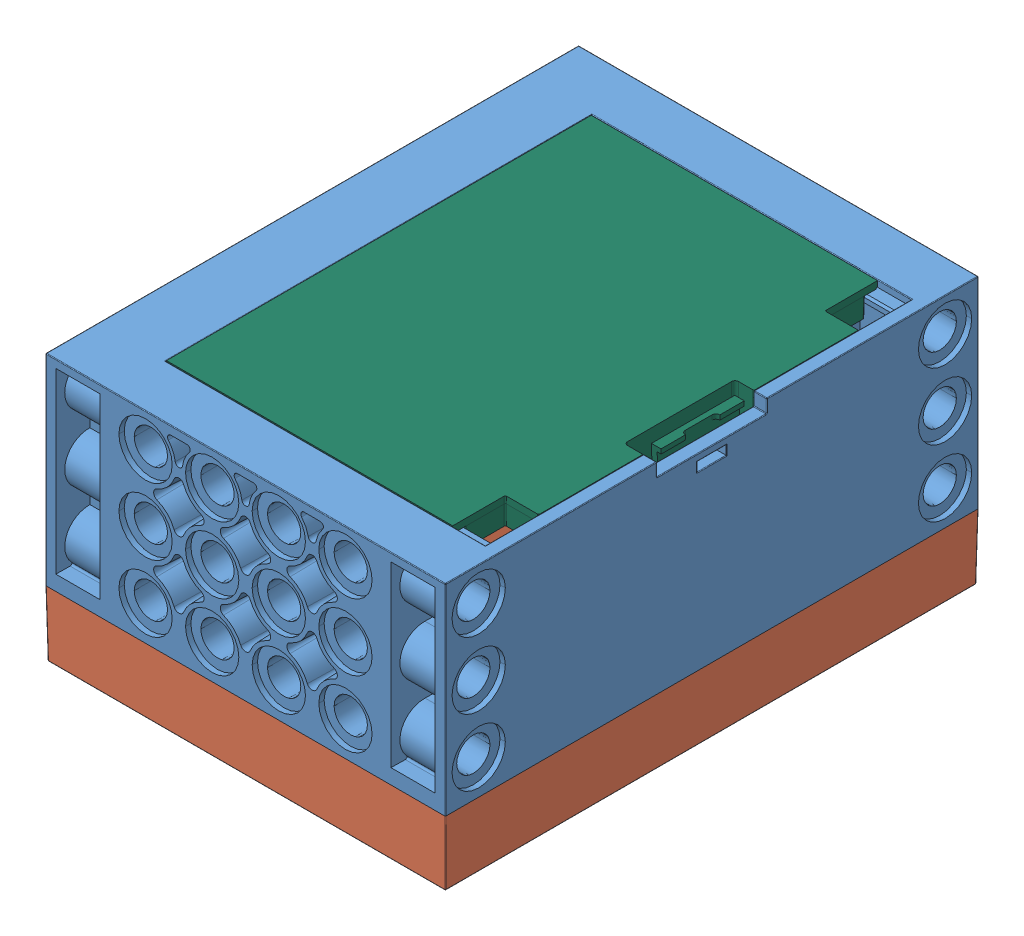
SolidWorks assembly BAbeta, configuration Default. Lengths in mm.
Overall size (60.01 40.02 80.01).
26 component instances, 15 part files, 0 mates.
Components (placement in the parent):
- babeta_0611-asm(2)^BAbeta-1: babeta_0611-asm(2)^BAbeta [Default] at origin size (60.01 40.02 80.01) (virtual)
  - BACA_ASSEMBLY_ASM_1LAST_VERSION_ASM^babeta_0611-asm(2)_BAbeta-1: BACA_ASSEMBLY_ASM_1LAST_VERSION_ASM^babeta_0611-asm(2)_BAbeta [Default] at origin size (60.01 40.02 80.01) (virtual)
    - BACA_ASM_2LAST_VERSION_ASM^BACA_ASSEMBLY_ASM_1LAST_VERSION_ASM_babeta_0611-asm(2)_BAbeta-1: BACA_ASM_2LAST_VERSION_ASM^BACA_ASSEMBLY_ASM_1LAST_VERSION_ASM_babeta_0611-asm(2)_BAbeta [Default] at origin size (60.01 40 80.01) (virtual)
      - BACA_1_27LAST_VERSION^BACA_ASM_2LAST_VERSION_ASM_BACA_ASSEMBLY_ASM_1LAST_VERSION_ASM_babeta_0611-asm(2)_BAbeta-1: BACA_1_27LAST_VERSION^BACA_ASM_2LAST_VERSION_ASM_BACA_ASSEMBLY_ASM_1LAST_VERSION_ASM_babeta_0611-asm(2)_BAbeta [Default] at origin size (60 31.6 80) (virtual)
      - BACA_2_25LAST_VERSION^BACA_ASM_2LAST_VERSION_ASM_BACA_ASSEMBLY_ASM_1LAST_VERSION_ASM_babeta_0611-asm(2)_BAbeta-1: BACA_2_25LAST_VERSION^BACA_ASM_2LAST_VERSION_ASM_BACA_ASSEMBLY_ASM_1LAST_VERSION_ASM_babeta_0611-asm(2)_BAbeta [Default] at origin size (60.01 12.3 80.01) (virtual)
    - BATTERY_HOLDER_WZY-148-1_WITH_C_ASM^BACA_ASSEMBLY_ASM_1LAST_VERSION_ASM_babeta_0611-asm(2)_BAbeta-1: BATTERY_HOLDER_WZY-148-1_WITH_C_ASM^BACA_ASSEMBLY_ASM_1LAST_VERSION_ASM_babeta_0611-asm(2)_BAbeta [Default] at (-86.1 17.025 0.8) x (1 0 0) z (0 0 -1) size (47.6 28.03 57.9) (virtual)
      - BATTERY_HOLDER_WZY-148-1_ASM^BATTERY_HOLDER_WZY-148-1_WITH_C_ASM_BACA_ASSEMBLY_ASM_1LAST_VERSION_ASM_babeta_0611-asm(2)_BAbeta-1: BATTERY_HOLDER_WZY-148-1_ASM^BATTERY_HOLDER_WZY-148-1_WITH_C_ASM_BACA_ASSEMBLY_ASM_1LAST_VERSION_ASM_babeta_0611-asm(2)_BAbeta [Default] at (0 0 28.6) size (47.6 28.03 57.9) (virtual)
        - SOLID1^BATTERY_HOLDER_WZY-148-1_ASM_BATTERY_HOLDER_WZY-148-1_WITH_C_ASM_BACA_ASSEMBLY_ASM_1LAST_VERSION_ASM_babeta_0611-asm(2)_BAbeta-1: SOLID1^BATTERY_HOLDER_WZY-148-1_ASM_BATTERY_HOLDER_WZY-148-1_WITH_C_ASM_BACA_ASSEMBLY_ASM_1LAST_VERSION_ASM_babeta_0611-asm(2)_BAbeta [Default] at origin size (47.6 14 57.9) (virtual)
        - SOLID2^BATTERY_HOLDER_WZY-148-1_ASM_BATTERY_HOLDER_WZY-148-1_WITH_C_ASM_BACA_ASSEMBLY_ASM_1LAST_VERSION_ASM_babeta_0611-asm(2)_BAbeta-1: SOLID2^BATTERY_HOLDER_WZY-148-1_ASM_BATTERY_HOLDER_WZY-148-1_WITH_C_ASM_BACA_ASSEMBLY_ASM_1LAST_VERSION_ASM_babeta_0611-asm(2)_BAbeta [Default] at origin size (10.31 10.11 8.59) (virtual)
        - SOLID3^BATTERY_HOLDER_WZY-148-1_ASM_BATTERY_HOLDER_WZY-148-1_WITH_C_ASM_BACA_ASSEMBLY_ASM_1LAST_VERSION_ASM_babeta_0611-asm(2)_BAbeta-1: SOLID3^BATTERY_HOLDER_WZY-148-1_ASM_BATTERY_HOLDER_WZY-148-1_WITH_C_ASM_BACA_ASSEMBLY_ASM_1LAST_VERSION_ASM_babeta_0611-asm(2)_BAbeta [Default] at origin size (10.31 10.11 8.59) (virtual)
        - SOLID4^BATTERY_HOLDER_WZY-148-1_ASM_BATTERY_HOLDER_WZY-148-1_WITH_C_ASM_BACA_ASSEMBLY_ASM_1LAST_VERSION_ASM_babeta_0611-asm(2)_BAbeta-1: SOLID4^BATTERY_HOLDER_WZY-148-1_ASM_BATTERY_HOLDER_WZY-148-1_WITH_C_ASM_BACA_ASSEMBLY_ASM_1LAST_VERSION_ASM_babeta_0611-asm(2)_BAbeta [Default] at origin size (7.96 7.79 6.52) (virtual)
        - SOLID5^BATTERY_HOLDER_WZY-148-1_ASM_BATTERY_HOLDER_WZY-148-1_WITH_C_ASM_BACA_ASSEMBLY_ASM_1LAST_VERSION_ASM_babeta_0611-asm(2)_BAbeta-1: SOLID5^BATTERY_HOLDER_WZY-148-1_ASM_BATTERY_HOLDER_WZY-148-1_WITH_C_ASM_BACA_ASSEMBLY_ASM_1LAST_VERSION_ASM_babeta_0611-asm(2)_BAbeta [Default] at origin size (5.15 13.26 53.2) (virtual)
        - SOLID6^BATTERY_HOLDER_WZY-148-1_ASM_BATTERY_HOLDER_WZY-148-1_WITH_C_ASM_BACA_ASSEMBLY_ASM_1LAST_VERSION_ASM_babeta_0611-asm(2)_BAbeta-1: SOLID6^BATTERY_HOLDER_WZY-148-1_ASM_BATTERY_HOLDER_WZY-148-1_WITH_C_ASM_BACA_ASSEMBLY_ASM_1LAST_VERSION_ASM_babeta_0611-asm(2)_BAbeta [Default] at origin size (5.15 13.26 53.2) (virtual)
        - SOLID10^BATTERY_HOLDER_WZY-148-1_ASM_BATTERY_HOLDER_WZY-148-1_WITH_C_ASM_BACA_ASSEMBLY_ASM_1LAST_VERSION_ASM_babeta_0611-asm(2)_BAbeta-1: SOLID10^BATTERY_HOLDER_WZY-148-1_ASM_BATTERY_HOLDER_WZY-148-1_WITH_C_ASM_BACA_ASSEMBLY_ASM_1LAST_VERSION_ASM_babeta_0611-asm(2)_BAbeta [Default] at origin size (5.15 13.26 53.2) (virtual)
        - SOLID11^BATTERY_HOLDER_WZY-148-1_ASM_BATTERY_HOLDER_WZY-148-1_WITH_C_ASM_BACA_ASSEMBLY_ASM_1LAST_VERSION_ASM_babeta_0611-asm(2)_BAbeta-1: SOLID11^BATTERY_HOLDER_WZY-148-1_ASM_BATTERY_HOLDER_WZY-148-1_WITH_C_ASM_BACA_ASSEMBLY_ASM_1LAST_VERSION_ASM_babeta_0611-asm(2)_BAbeta [Default] at origin size (5.15 13.26 53.2) (virtual)
        - SOLID13^BATTERY_HOLDER_WZY-148-1_ASM_BATTERY_HOLDER_WZY-148-1_WITH_C_ASM_BACA_ASSEMBLY_ASM_1LAST_VERSION_ASM_babeta_0611-asm(2)_BAbeta-1: SOLID13^BATTERY_HOLDER_WZY-148-1_ASM_BATTERY_HOLDER_WZY-148-1_WITH_C_ASM_BACA_ASSEMBLY_ASM_1LAST_VERSION_ASM_babeta_0611-asm(2)_BAbeta [Default] at origin size (47.6 14 57.9) (virtual)
        - SOLID16^BATTERY_HOLDER_WZY-148-1_ASM_BATTERY_HOLDER_WZY-148-1_WITH_C_ASM_BACA_ASSEMBLY_ASM_1LAST_VERSION_ASM_babeta_0611-asm(2)_BAbeta-1: SOLID16^BATTERY_HOLDER_WZY-148-1_ASM_BATTERY_HOLDER_WZY-148-1_WITH_C_ASM_BACA_ASSEMBLY_ASM_1LAST_VERSION_ASM_babeta_0611-asm(2)_BAbeta [Default] at origin size (10.32 10.11 8.61) (virtual)
        - SOLID17^BATTERY_HOLDER_WZY-148-1_ASM_BATTERY_HOLDER_WZY-148-1_WITH_C_ASM_BACA_ASSEMBLY_ASM_1LAST_VERSION_ASM_babeta_0611-asm(2)_BAbeta-1: SOLID17^BATTERY_HOLDER_WZY-148-1_ASM_BATTERY_HOLDER_WZY-148-1_WITH_C_ASM_BACA_ASSEMBLY_ASM_1LAST_VERSION_ASM_babeta_0611-asm(2)_BAbeta [Default] at origin size (10.32 10.11 8.61) (virtual)
        - SOLID18^BATTERY_HOLDER_WZY-148-1_ASM_BATTERY_HOLDER_WZY-148-1_WITH_C_ASM_BACA_ASSEMBLY_ASM_1LAST_VERSION_ASM_babeta_0611-asm(2)_BAbeta-1: SOLID18^BATTERY_HOLDER_WZY-148-1_ASM_BATTERY_HOLDER_WZY-148-1_WITH_C_ASM_BACA_ASSEMBLY_ASM_1LAST_VERSION_ASM_babeta_0611-asm(2)_BAbeta [Default] at origin size (10.24 10.11 8.59) (virtual)
      - BATTERY^BATTERY_HOLDER_WZY-148-1_WITH_C_ASM_BACA_ASSEMBLY_ASM_1LAST_VERSION_ASM_babeta_0611-asm(2)_BAbeta-1: BATTERY^BATTERY_HOLDER_WZY-148-1_WITH_C_ASM_BACA_ASSEMBLY_ASM_1LAST_VERSION_ASM_babeta_0611-asm(2)_BAbeta [Default] at (0 8.075 -24.04) x (0.984229 0.176899 0) z (0 0 1) (virtual)
      - BATTERY^BATTERY_HOLDER_WZY-148-1_WITH_C_ASM_BACA_ASSEMBLY_ASM_1LAST_VERSION_ASM_babeta_0611-asm(2)_BAbeta-2: BATTERY^BATTERY_HOLDER_WZY-148-1_WITH_C_ASM_BACA_ASSEMBLY_ASM_1LAST_VERSION_ASM_babeta_0611-asm(2)_BAbeta [Default] at (15.25 8.075 24.1901) x (0.978701 0.205292 0) z (0 0 -1) (virtual)
      - BATTERY^BATTERY_HOLDER_WZY-148-1_WITH_C_ASM_BACA_ASSEMBLY_ASM_1LAST_VERSION_ASM_babeta_0611-asm(2)_BAbeta-3: BATTERY^BATTERY_HOLDER_WZY-148-1_WITH_C_ASM_BACA_ASSEMBLY_ASM_1LAST_VERSION_ASM_babeta_0611-asm(2)_BAbeta [Default] at (0 -8.075 24.04) x (-0.240038 0.970763 0) z (0 0 -1) (virtual)
      - BATTERY^BATTERY_HOLDER_WZY-148-1_WITH_C_ASM_BACA_ASSEMBLY_ASM_1LAST_VERSION_ASM_babeta_0611-asm(2)_BAbeta-4: BATTERY^BATTERY_HOLDER_WZY-148-1_WITH_C_ASM_BACA_ASSEMBLY_ASM_1LAST_VERSION_ASM_babeta_0611-asm(2)_BAbeta [Default] at (15.25 -8.075 -24.1901) x (0.189266 0.981926 0) z (0 0 1) (virtual)
      - BATTERY^BATTERY_HOLDER_WZY-148-1_WITH_C_ASM_BACA_ASSEMBLY_ASM_1LAST_VERSION_ASM_babeta_0611-asm(2)_BAbeta-5: BATTERY^BATTERY_HOLDER_WZY-148-1_WITH_C_ASM_BACA_ASSEMBLY_ASM_1LAST_VERSION_ASM_babeta_0611-asm(2)_BAbeta [Default] at (-15.25 -8.075 -24.1901) x (-0.999814 -0.019277 0) z (0 0 1) (virtual)
      - BATTERY^BATTERY_HOLDER_WZY-148-1_WITH_C_ASM_BACA_ASSEMBLY_ASM_1LAST_VERSION_ASM_babeta_0611-asm(2)_BAbeta-6: BATTERY^BATTERY_HOLDER_WZY-148-1_WITH_C_ASM_BACA_ASSEMBLY_ASM_1LAST_VERSION_ASM_babeta_0611-asm(2)_BAbeta [Default] at (-15.25 8.075 24.1901) x (0.546844 0.837235 0) z (0 0 -1) (virtual)
    - BACA_3^BACA_ASSEMBLY_ASM_1LAST_VERSION_ASM_babeta_0611-asm(2)_BAbeta-1: BACA_3^BACA_ASSEMBLY_ASM_1LAST_VERSION_ASM_babeta_0611-asm(2)_BAbeta [Default] at (-86 38 0) x (1 0 0) z (0 1 0) size (50.2 63.79 10.03) (virtual)
